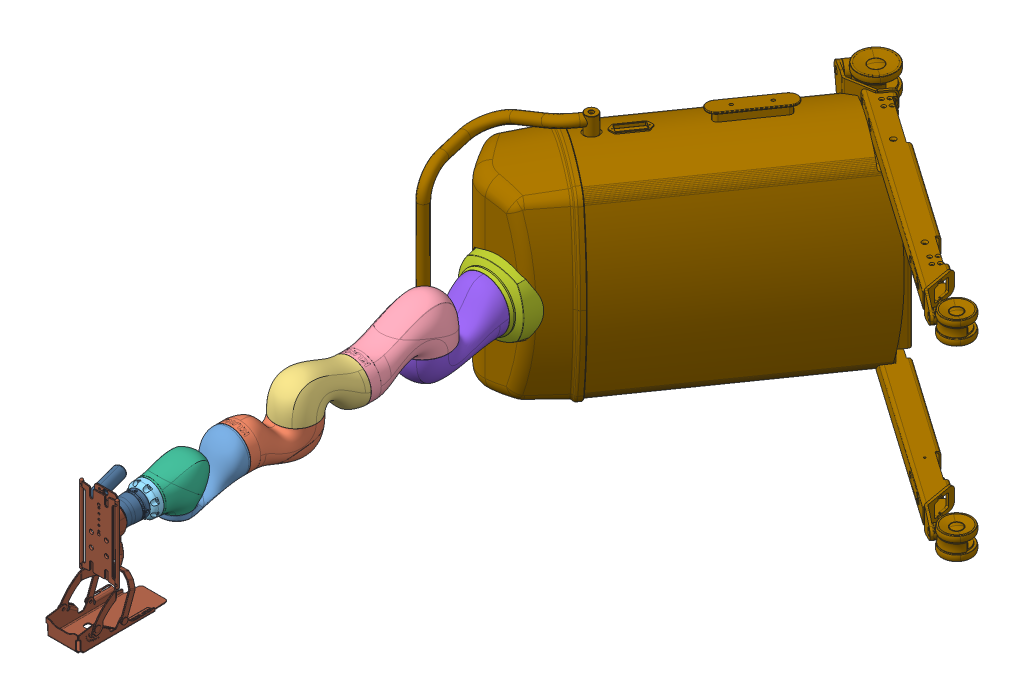
SolidWorks assembly lbrMed_withBaseLink_FramesBase, configuration Default. Lengths in mm.
Overall size (1621.06 766 2493.59).
11 component instances, 11 part files, 10 mates.
Components (placement in the parent):
- Wrist1_body-2: Wrist1_body [Default] at origin size (137.43 170.81 261.47)
- UpperArm_body-1: UpperArm_body [Default] at origin size (137.03 183.96 286.04)
- Elbow_body-1: Elbow_body [Default] at origin size (136.09 183.95 261.22)
- LowerArm_body-1: LowerArm_body [Default] at origin size (171.08 201.65 323.93)
- Wrist3_body-1: Wrist3_body [Default] at origin size (102.25 102.25 38.4)
- Wrist2_body-1: Wrist2_body [Default] at origin size (136.25 137.94 182.79)
- Base_body-1: Base_body [Default] at origin size (277.84 277.84 157.78)
- Shoulder_body-1: Shoulder_body [Default] at origin size (171.08 202.96 299.34)
- only_platform-1: only_platform [Default] at (515.1468 0 -732.7058) x (-0.819152 0 -0.573576) z (0 1 0) size (1151.95 1181.08 766)
- only_link-1: only_link [Default] at (515.1468 0 -732.7058) x (-0.819152 0 -0.573576) z (0 1 0) size (221.89 131.55 78.48)
- boot-1: boot [Default] at (0 -29.8592 1410.13) x (0 -1 0) z (1 0 0) size (394.15 308.25 145.27)
Mates (geometry in assembly coordinates):
- Concentric1: concentric aligned: cylinder of Base_body-1 through (84.8528 84.8528 0) axis (0 0 1) radius 5; cylinder of only_platform-1 through (84.8528 84.8528 -125.779) axis (0 0 1) radius 5.25
- Concentric2: concentric aligned: cylinder of Base_body-1 through (84.8528 -84.8528 0) axis (0 0 1) radius 5; cylinder of only_platform-1 through (84.8528 -84.8528 -125.779) axis (0 0 1) radius 5.25
- Coincident1: coincident anti-aligned: plane of Base_body-1 through (0 0 3) normal (0 0 -1); plane of only_platform-1 through (127.5 127.5 3) normal (0 0 1)
- Concentric3: concentric anti-aligned: cylinder of Wrist3_body-1 through (-9.7581 9.7581 1289.3) axis (0 0 1) radius 3.2; cylinder of only_link-1 through (-9.7581 9.7581 1305.98) axis (0 0 -1) radius 3.2
- Concentric4: concentric anti-aligned: cylinder of Wrist3_body-1 through (9.7581 -9.7581 1289.3) axis (0 0 1) radius 3.2; cylinder of only_link-1 through (9.7581 -9.7581 1305.98) axis (0 0 -1) radius 3.2
- Coincident2: coincident anti-aligned: plane of Wrist3_body-1 through (0 30.5 1306) normal (0 0 1); plane of only_link-1 through (0 0 1306) normal (0 0 -1)
- Coincident3: coincident: plane of only_link-1 through (0 0 1392.13) normal (0 0 1); plane of boot-1 through (0 0 1392.13) normal (0 0 -1)
- Concentric5: concentric: circle of only_link-1; circle of boot-1
- Parallel4: parallel: cylinder of only_link-1 through (-0.1001 -36.0999 1226.8324) axis (0 0 -1) radius 1; cylinder of boot-1 through (0.6001 -37.9953 1378.63) axis (0 0 -1) radius 1.1
- Parallel5: parallel aligned: plane of only_link-1 through (-13.6777 -20 1346.48) normal (1 0 0); plane of boot-1 through (-10.3 0 1405.13) normal (1 0 0)
